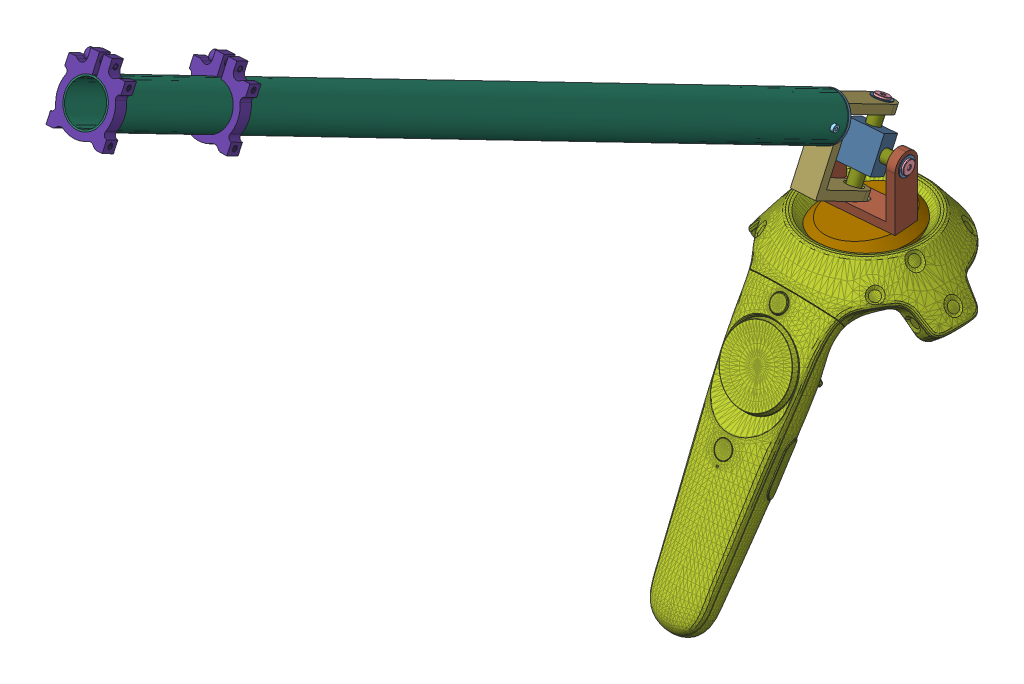
SolidWorks assembly WandMountCAl, configuration Default. Lengths in mm.
Overall size (118.5 507.84 533.23).
33 component instances, 17 part files, 72 mates.
Components (placement in the parent):
- 57155K301_Stainless Steel Ball BearingBAl-5: 57155K301_Stainless Steel Ball BearingBAl [57155K301] at (0 1.0795 0) x (-0.199974 0 0.979801) z (0 1 0) size (10.72 10.72 3.17)
- 57155K301_Stainless Steel Ball BearingBAl-6: 57155K301_Stainless Steel Ball BearingBAl [57155K301] at (0 13.9205 0) x (0.455162 0 -0.890409) z (0 -1 0) size (10.72 10.72 3.17)
- 91251A196_Black-Oxide Alloy Steel Socket Head ScrewAl-1: 91251A196_Black-Oxide Alloy Steel Socket Head ScrewAl [91251A196] at (0 -5.6453 12.5) x (0.587183 0 -0.809454) z (0 -1 0) size (6.86 6.86 20.6)
- 91251A196_Black-Oxide Alloy Steel Socket Head ScrewAl-2: 91251A196_Black-Oxide Alloy Steel Socket Head ScrewAl [91251A196] at (0 -5.6453 -12.5) x (0.424116 0 -0.905608) z (0 -1 0) size (6.86 6.86 20.6)
- 92012A207_Alloy Steel Precision Shoulder ScrewAl-1: 92012A207_Alloy Steel Precision Shoulder ScrewAl [92012A207] at (0 -6.0643 0) x (0.734602 0 0.678499) z (0 -1 0) size (7.94 7.94 28.23)
- 57155K301_Stainless Steel Ball BearingBAl-7: 57155K301_Stainless Steel Ball BearingBAl [57155K301] at (21.3447 48.8017 -1.7999) x (-0.030138 -0.933464 -0.357402) z (-0.996464 0 0.084026) size (10.72 10.72 3.17)
- 57155K301_Stainless Steel Ball BearingBAl-8: 57155K301_Stainless Steel Ball BearingBAl [57155K301] at (0.8273 29.7783 9.8114) x (-0.627222 -0.378377 -0.680752) z (-0.038623 0.888094 -0.458036) size (10.72 10.72 3.17)
- 57155K301_Stainless Steel Ball BearingBAl-9: 57155K301_Stainless Steel Ball BearingBAl [57155K301] at (-21.3447 48.8017 1.7999) x (-0.082588 -0.184207 -0.979412) z (0.996464 0 -0.084026) size (10.72 10.72 3.17)
- 57155K301_Stainless Steel Ball BearingBAl-10: 57155K301_Stainless Steel Ball BearingBAl [57155K301] at (-0.8273 67.8252 -9.8114) x (0.991908 -0.021405 -0.125143) z (0.038623 -0.888094 0.458036) size (10.72 10.72 3.17)
- 90318A302_Ultra-Low-Profile Precision Shoulder ScrewAl-1: 90318A302_Ultra-Low-Profile Precision Shoulder ScrewAl [90318A302] at (-24.113 48.8017 2.0333) x (0.034978 -0.909239 0.414801) z (-0.996464 0 0.084026) size (7.94 7.94 15.93)
- 90318A302_Ultra-Low-Profile Precision Shoulder ScrewAl-2: 90318A302_Ultra-Low-Profile Precision Shoulder ScrewAl [90318A302] at (0.9346 27.3111 11.0839) x (-0.528864 0.370748 0.763445) z (0.038623 -0.888094 0.458036) size (7.94 7.94 15.93)
- 90318A302_Ultra-Low-Profile Precision Shoulder ScrewAl-3: 90318A302_Ultra-Low-Profile Precision Shoulder ScrewAl [90318A302] at (24.113 48.8017 -2.0333) x (0.083807 0.072112 0.993869) z (0.996464 0 -0.084026) size (7.94 7.94 15.93)
- 90318A302_Ultra-Low-Profile Precision Shoulder ScrewAl-4: 90318A302_Ultra-Low-Profile Precision Shoulder ScrewAl [90318A302] at (-0.9346 70.2924 -11.0839) x (0.980778 -0.054045 -0.187492) z (-0.038623 0.888094 -0.458036) size (7.94 7.94 15.93)
- 91290A015_Black-Oxide Alloy Steel Socket Head ScrewAl-1: 91290A015_Black-Oxide Alloy Steel Socket Head ScrewAl [91290A015] at (9.1737 81.0482 32.3414) x (-0.036412 0.683823 -0.728739) z (0.999254 0.034314 -0.017729) size (3.8 3.8 10.09)
- 91290A015_Black-Oxide Alloy Steel Socket Head ScrewAl-2: 91290A015_Black-Oxide Alloy Steel Socket Head ScrewAl [91290A015] at (-10.2118 80.3825 32.6853) x (-0.0328 0.511547 -0.858629) z (-0.999254 -0.034314 0.017729) size (3.8 3.8 10.09)
- 91251A192_Black-Oxide Alloy Steel Socket Head Screw-1: 91251A192_Black-Oxide Alloy Steel Socket Head Screw [91251A192] at (-0.5194 74.5981 20.6527) x (-0.99894 -0.040898 0.021125) z (-0.000028 -0.458379 -0.888757) size (6.86 6.86 14.21)
- Vive Controller 1.5BAl-1: Vive Controller 1.5BAl [Default] at (0.0016 6.0546 36.5874) x (1 -0.000227 0) z (-0.000192 -0.847056 0.531504) size (118.44 84.37 219.45)
- BottomPlugBAl-2: BottomPlugBAl [Default] at origin size (42.24 11.38 42.24)
- TopPlugBAl-2: TopPlugBAl [Default] at origin size (50.17 16.12 56.99)
- CrossAl-1: CrossAl [Default] at (0 48.8017 0) x (-0.996464 0 0.084026) z (0.038623 -0.888094 0.458036) size (20 10 20)
- FORKAl-1: FORKAl [Default] at (0 48.8017 0) x (-0.996464 0 0.084026) z (0 1 0) size (45 15 40)
- ForkTopAl-2: ForkTopAl [Default] at (0 48.8017 0) x (0.038623 -0.888094 0.458036) z (-0.000028 -0.458379 -0.888757) size (45 15 40)
- GimbalSpacerP3BAl-9: GimbalSpacerP3BAl [Default] at (0 -1.3017 0) x (0 1 0) z (0.815244 0 -0.579118) size (0.79 8 8)
- GimbalSpacerP3BAl-10: GimbalSpacerP3BAl [Default] at (0 -2.0955 0) x (0 1 0) z (0.691499 0 -0.722378) size (0.79 8 8)
- GimbalSpacerP3BAl-11: GimbalSpacerP3BAl [Default] at (0 15.508 0) x (0 1 0) z (0.519515 0 -0.854462) size (0.79 8 8)
- GimbalPlugP3CAl-1: GimbalPlugP3CAl [Default] at (-0.5194 75.6617 22.7148) x (-0.999254 -0.034314 0.017729) z (-0.038623 0.888094 -0.458036) size (25.4 16.5 25.4)
- MainTubeP3Al-1: MainTubeP3Al [Default] at (-0.5193 76.5899 24.5146) x (0.999254 0.034314 -0.017729) z (0.000028 0.458379 0.888757) size (25.4 25.4 504.28)
- CrossSpacer-1: CrossSpacer [Default] at (15.0172 48.8017 -1.2663) x (0.996464 0 -0.084026) z (0.084024 -0.005908 0.996446) size (9.53 7.14 7.14)
- CrossSpacer-2: CrossSpacer [Default] at (-15.0172 48.8017 1.2663) x (-0.996464 0 0.084026) z (-0.01061 0.991996 -0.12582) size (9.53 7.14 7.14)
- CrossSpacer-4: CrossSpacer [Default] at (-0.5821 62.1858 -6.9028) x (-0.038623 0.888094 -0.458036) z (0.818712 0.290928 0.495048) size (9.53 7.14 7.14)
- CrossSpacer-6: CrossSpacer [Default] at (0.5821 35.4177 6.9028) x (0.038623 -0.888094 0.458036) z (-0.347024 0.417928 0.839589) size (9.53 7.14 7.14)
- 545680P3-1: 545680P3 [Default] at (-0.1291 309.2768 462.1783) x (-0.999254 -0.034314 0.017729) z (0.038623 -0.888094 0.458036) size (33.53 7.62 39.7)
- 545680P3-2: 545680P3 [Default] at (-0.1315 270.3145 386.634) x (-0.999254 -0.034314 0.017729) z (0.038623 -0.888094 0.458036) size (33.53 7.62 39.7)
Mates (geometry in assembly coordinates):
- Coincident5: coincident aligned: plane of Vive Controller 1.5-1 through (0.0016 0 36.5874) normal (0 1 0)
- Coincident4: coordinate: point of BottomPlug-2
- Coincident6: coincident: line of Vive Controller 1.5-1 through (0 0 0) axis (0 1 0)
- Coincident7: coincident: line of Vive Controller 1.5-1 through (0 0 0) axis (0 1 0)
- Parallel1: parallel anti-aligned: plane of Vive Controller 1.5-1 through (0.0016 6.0546 -0.0032) normal (0 0 -1)
- Coincident9: coordinate: unknown of TopPlugB-2
- Concentric45: concentric aligned: cylinder of 57155K301_Stainless Steel Ball BearingB-5 through (0 1.0795 0) axis (0 1 0) radius 2.3813; cylinder of 92012A207_Alloy Steel Precision Shoulder ScrewAl-1 through (0 21.717 0) axis (0 1 0) radius 2.3813
- Concentric47: concentric anti-aligned: cylinder of 57155K301_Stainless Steel Ball BearingB-6 through (0 13.9205 0) axis (0 -1 0) radius 2.3813; cylinder of 92012A207_Alloy Steel Precision Shoulder ScrewAl-1 through (0 21.717 0) axis (0 1 0) radius 2.3813
- Concentric56: concentric anti-aligned: cylinder of TopPlugB-2 through (0 3.5 0) axis (0 -1 0) radius 4.7625; cylinder of 57155K301_Stainless Steel Ball BearingB-5 through (0 1.0795 0) axis (0 1 0) radius 4.7625
- Coincident41: coincident anti-aligned: plane of TopPlugB-2 through (0 0 0) normal (0 -1 0); plane of 57155K301_Stainless Steel Ball BearingB-5 through (5.2511 0 1.0717) normal (0 1 0)
- Concentric57: concentric anti-aligned: cylinder of TopPlugB-2 through (0 11.5 0) axis (0 1 0) radius 4.7625; cylinder of 57155K301_Stainless Steel Ball BearingB-6 through (0 13.9205 0) axis (0 -1 0) radius 4.7625
- Coincident42: coincident anti-aligned: plane of TopPlugB-2 through (0 15 0) normal (0 1 0); plane of 57155K301_Stainless Steel Ball BearingB-6 through (4.7721 15 2.4394) normal (0 -1 0)
- Concentric63: concentric anti-aligned: cylinder of BottomPlugB-2 through (0 -11.5 12.5) axis (0 -1 0) radius 2.2479; cylinder of 91251A196_Black-Oxide Alloy Steel Socket Head Screw-1 through (0 4.375 12.5) axis (0 1 0) radius 3.429
- Coincident43: coincident anti-aligned: plane of BottomPlugB-2 through (0 -11.5 0) normal (0 -1 0); plane of 91251A196_Black-Oxide Alloy Steel Socket Head Screw-1 through (2.4384 -11.5 14.2689) normal (0 1 0)
- Concentric64: concentric anti-aligned: cylinder of BottomPlugB-2 through (0 -11.5 -12.5) axis (0 -1 0) radius 2.2479; cylinder of 91251A196_Black-Oxide Alloy Steel Socket Head Screw-2 through (0 4.375 -12.5) axis (0 1 0) radius 3.429
- Coincident44: coincident anti-aligned: plane of BottomPlugB-2 through (0 -11.5 0) normal (0 -1 0); plane of 91251A196_Black-Oxide Alloy Steel Socket Head Screw-2 through (2.7281 -11.5 -11.2224) normal (0 1 0)
- Width1: width anti-aligned: plane of FORKAl-1 through (-16.8079 56.3017 8.9439) normal (0.996464 0 -0.084026); plane of FORKAl-1 through (18.0683 21.3018 6.003) normal (-0.996464 0 0.084026); plane of CrossAl-1 through (-10.3377 46.5034 -3.5845) normal (-0.996464 0 0.084026); plane of CrossAl-1 through (9.5915 46.5034 -5.265) normal (0.996464 0 -0.084026)
- Width2: width aligned: plane of ForkTopAl-2 through (-8.1695 76.6915 16.5581) normal (0.038623 -0.888094 0.458036); plane of ForkTopAl-2 through (-6.8187 29.5649 1.4829) normal (-0.038623 0.888094 -0.458036); plane of CrossAl-1 through (0.0131 37.6225 0.1556) normal (0.038623 -0.888094 0.458036); plane of CrossAl-1 through (-0.7593 55.3844 -9.0051) normal (-0.038623 0.888094 -0.458036)
- Concentric7: concentric aligned: cylinder of FORKAl-1 through (22.4204 48.8017 -1.8906) axis (-0.996464 0 0.084026) radius 4.7625; cylinder of 57155K301_Stainless Steel Ball BearingBAl-7 through (21.3447 48.8017 -1.7999) axis (-0.996464 0 0.084026) radius 4.7625
- Coincident10: coincident anti-aligned: plane of FORKAl-1 through (23.0506 56.3017 5.5829) normal (0.996464 0 -0.084026); plane of 57155K301_Stainless Steel Ball BearingBAl-7 through (22.8408 46.8795 3.0945) normal (-0.996464 0 0.084026)
- Concentric9: concentric anti-aligned: cylinder of FORKAl-1 through (22.4204 48.8017 -1.8906) axis (-0.996464 0 0.084026) radius 4.7625; cylinder of 57155K301_Stainless Steel Ball BearingBAl-9 through (-21.3447 48.8017 1.7999) axis (0.996464 0 -0.084026) radius 4.7625
- Coincident12: coincident anti-aligned: plane of FORKAl-1 through (-21.7902 16.3018 9.3641) normal (-0.996464 0 0.084026); plane of 57155K301_Stainless Steel Ball BearingBAl-9 through (-22.5034 54.0694 0.9068) normal (0.996464 0 -0.084026)
- Concentric8: concentric anti-aligned: cylinder of ForkTopAl-2 through (-0.869 68.7839 -10.3058) axis (0.038623 -0.888094 0.458036) radius 4.7625; cylinder of 57155K301_Stainless Steel Ball BearingBAl-8 through (0.8273 29.7783 9.8114) axis (-0.038623 0.888094 -0.458036) radius 4.7625
- Coincident11: coincident anti-aligned: plane of ForkTopAl-2 through (-6.6245 43.4596 39.3234) normal (0.038623 -0.888094 0.458036); plane of 57155K301_Stainless Steel Ball BearingBAl-8 through (-3.3 30.2184 13.3695) normal (-0.038623 0.888094 -0.458036)
- Concentric10: concentric aligned: cylinder of ForkTopAl-2 through (-0.869 68.7839 -10.3058) axis (0.038623 -0.888094 0.458036) radius 4.7625; cylinder of 57155K301_Stainless Steel Ball BearingBAl-10 through (-0.8273 67.8252 -9.8114) axis (0.038623 -0.888094 0.458036) radius 4.7625
- Coincident13: coincident anti-aligned: plane of ForkTopAl-2 through (-8.3636 65.0887 -16.8385) normal (-0.038623 0.888094 -0.458036); plane of 57155K301_Stainless Steel Ball BearingBAl-10 through (-0.2208 71.2447 -5.5891) normal (0.038623 -0.888094 0.458036)
- Concentric15: concentric aligned: cylinder of 57155K301_Stainless Steel Ball BearingBAl-7 through (21.3447 48.8017 -1.7999) axis (-0.996464 0 0.084026) radius 2.3813; cylinder of 90318A302_Ultra-Low-Profile Precision Shoulder ScrewAl-3 through (8.6897 48.8017 -0.7327) axis (-0.996464 0 0.084026) radius 2.3813
- Coincident16: coincident anti-aligned: plane of 57155K301_Stainless Steel Ball BearingBAl-7 through (23.1694 47.6914 0.9462) normal (0.996464 0 -0.084026); plane of 90318A302_Ultra-Low-Profile Precision Shoulder ScrewAl-3 through (22.9026 52.7602 -2.2184) normal (-0.996464 0 0.084026)
- Concentric13: concentric aligned: cylinder of 57155K301_Stainless Steel Ball BearingBAl-8 through (0.8273 29.7783 9.8114) axis (-0.038623 0.888094 -0.458036) radius 2.3813; cylinder of 90318A302_Ultra-Low-Profile Precision Shoulder ScrewAl-2 through (0.3368 41.0571 3.9943) axis (-0.038623 0.888094 -0.458036) radius 2.3813
- Coincident15: coincident anti-aligned: plane of 57155K301_Stainless Steel Ball BearingBAl-8 through (-1.5194 29.1764 12.3081) normal (0.038623 -0.888094 0.458036); plane of 90318A302_Ultra-Low-Profile Precision Shoulder ScrewAl-2 through (4.2535 29.4469 12.3457) normal (-0.038623 0.888094 -0.458036)
- Concentric11: concentric aligned: cylinder of 57155K301_Stainless Steel Ball BearingBAl-9 through (-21.3447 48.8017 1.7999) axis (0.996464 0 -0.084026) radius 2.3813; cylinder of 90318A302_Ultra-Low-Profile Precision Shoulder ScrewAl-1 through (-8.6897 48.8017 0.7327) axis (0.996464 0 -0.084026) radius 2.3813
- Coincident14: coincident anti-aligned: plane of 57155K301_Stainless Steel Ball BearingBAl-9 through (-22.9745 51.8444 1.365) normal (-0.996464 0 0.084026); plane of 90318A302_Ultra-Low-Profile Precision Shoulder ScrewAl-1 through (-23.2298 47.1497 -1.6625) normal (0.996464 0 -0.084026)
- Concentric17: concentric aligned: cylinder of 57155K301_Stainless Steel Ball BearingBAl-10 through (-0.8273 67.8252 -9.8114) axis (0.038623 -0.888094 0.458036) radius 2.3813; cylinder of 90318A302_Ultra-Low-Profile Precision Shoulder ScrewAl-4 through (-0.3368 56.5464 -3.9943) axis (0.038623 -0.888094 0.458036) radius 2.3813
- Coincident17: coincident anti-aligned: plane of 57155K301_Stainless Steel Ball BearingBAl-10 through (-0.5143 70.6564 -7.8141) normal (-0.038623 0.888094 -0.458036); plane of 90318A302_Ultra-Low-Profile Precision Shoulder ScrewAl-4 through (-0.1296 71.0466 -7.0899) normal (0.038623 -0.888094 0.458036)
- Concentric68: concentric anti-aligned: cylinder of 92012A207_Alloy Steel Precision Shoulder ScrewAl-1 through (0 21.717 0) axis (0 1 0) radius 2.3813; cylinder of GimbalSpacerP3BAl-9 through (0 -0.508 0) axis (0 -1 0) radius 2.3813
- Coincident48: coincident anti-aligned: plane of 57155K301_Stainless Steel Ball BearingB-5 through (3.0331 -0.508 0.619) normal (0 -1 0); plane of GimbalSpacerP3BAl-9 through (0 -0.508 0) normal (0 1 0)
- Concentric69: concentric anti-aligned: cylinder of 92012A207_Alloy Steel Precision Shoulder ScrewAl-1 through (0 21.717 0) axis (0 1 0) radius 2.3813; cylinder of GimbalSpacerP3BAl-10 through (0 -1.3017 0) axis (0 -1 0) radius 2.3813
- Coincident49: coincident anti-aligned: plane of GimbalSpacerP3BAl-9 through (0 -1.3017 0) normal (0 -1 0); plane of GimbalSpacerP3BAl-10 through (0 -1.3017 0) normal (0 1 0)
- Concentric70: concentric anti-aligned: cylinder of 92012A207_Alloy Steel Precision Shoulder ScrewAl-1 through (0 21.717 0) axis (0 1 0) radius 2.3813; cylinder of GimbalSpacerP3BAl-11 through (0 16.3018 0) axis (0 -1 0) radius 2.3813
- Coincident51: coincident anti-aligned: plane of 92012A207_Alloy Steel Precision Shoulder ScrewAl-1 through (2.6928 -2.0955 -2.9155) normal (0 1 0); plane of GimbalSpacerP3BAl-10 through (0 -2.0955 0) normal (0 -1 0)
- Coincident52: coincident anti-aligned: plane of 57155K301_Stainless Steel Ball BearingB-6 through (2.7564 15.508 1.409) normal (0 1 0); plane of GimbalSpacerP3BAl-11 through (0 15.508 0) normal (0 -1 0)
- Coincident56: coincident anti-aligned: plane of ForkTopAl-2 through (-8.3625 83.4238 18.7117) normal (0.000028 0.458379 0.888757); plane of GimbalPlugP3CAl-1 through (-1.0099 86.9405 16.8978) normal (-0.000028 -0.458379 -0.888757)
- Coincident62: coincident aligned: axis of 91290A015_Black-Oxide Alloy Steel Socket Head ScrewAl-2 through (-13.2096 80.2796 32.7385) axis (0.999254 0.034314 -0.017729); line of MainTubeP3Al-1 through (-13.2096 80.2796 32.7385) axis (0.999254 0.034314 -0.017729)
- Coincident63: coincident aligned: line of GimbalPlugP3CAl-1 through (-0.5189 83.225 37.3793) axis (-0.000028 -0.458379 -0.888757); line of MainTubeP3Al-1 through (-0.5052 307.7415 472.6967) axis (-0.000028 -0.458379 -0.888757)
- Tangent4: tangent anti-aligned: plane of 91290A015_Black-Oxide Alloy Steel Socket Head ScrewAl-1 through (12.1483 82.463 33.5204) normal (-0.999254 -0.034314 0.017729); cylinder of MainTubeP3Al-1 through (-0.5052 307.7415 472.6967) axis (-0.000028 -0.458379 -0.888757) radius 12.7
- Tangent5: tangent anti-aligned: plane of 91290A015_Black-Oxide Alloy Steel Socket Head ScrewAl-2 through (-13.1729 78.7341 31.8164) normal (0.999254 0.034314 -0.017729); cylinder of MainTubeP3Al-1 through (-0.5052 307.7415 472.6967) axis (-0.000028 -0.458379 -0.888757) radius 12.7
- Concentric73: concentric anti-aligned: cylinder of 90318A302_Ultra-Low-Profile Precision Shoulder ScrewAl-1 through (-8.6897 48.8017 0.7327) axis (0.996464 0 -0.084026) radius 2.3813; cylinder of CrossAl-1 through (-9.9646 48.8017 0.8403) axis (-0.996464 0 0.084026) radius 1.7272
- Concentric74: concentric anti-aligned: cylinder of 90318A302_Ultra-Low-Profile Precision Shoulder ScrewAl-3 through (8.6897 48.8017 -0.7327) axis (-0.996464 0 0.084026) radius 2.3813; cylinder of CrossAl-1 through (9.9646 48.8017 -0.8403) axis (0.996464 0 -0.084026) radius 1.7272
- Concentric75: concentric anti-aligned: cylinder of 90318A302_Ultra-Low-Profile Precision Shoulder ScrewAl-2 through (0.3368 41.0571 3.9943) axis (-0.038623 0.888094 -0.458036) radius 2.3813; cylinder of CrossAl-1 through (0.3862 39.9208 4.5804) axis (0.038623 -0.888094 0.458036) radius 1.7272
- Concentric76: concentric anti-aligned: cylinder of 90318A302_Ultra-Low-Profile Precision Shoulder ScrewAl-4 through (-0.3368 56.5464 -3.9943) axis (0.038623 -0.888094 0.458036) radius 2.3813; cylinder of CrossAl-1 through (-0.3862 57.6827 -4.5804) axis (-0.038623 0.888094 -0.458036) radius 1.7272
- Concentric77: concentric aligned: cylinder of ForkTopAl-2 through (-0.5195 73.3698 18.2711) axis (-0.000028 -0.458379 -0.888757) radius 1.7272; cylinder of GimbalPlugP3CAl-1 through (-0.5472 -382.7178 -866.0417) axis (-0.000028 -0.458379 -0.888757) radius 2.8067
- Concentric78: concentric anti-aligned: cylinder of GimbalPlugP3CAl-1 through (-11.6233 80.334 32.7104) axis (-0.999254 -0.034314 0.017729) radius 1.25; cylinder of 91290A015_Black-Oxide Alloy Steel Socket Head ScrewAl-2 through (-5.2155 80.5541 32.5967) axis (0.999254 0.034314 -0.017729) radius 1.9
- Concentric79: concentric anti-aligned: cylinder of GimbalPlugP3CAl-1 through (10.5852 81.0967 32.3164) axis (0.999254 0.034314 -0.017729) radius 1.25; cylinder of 91290A015_Black-Oxide Alloy Steel Socket Head ScrewAl-1 through (4.1774 80.8766 32.4301) axis (-0.999254 -0.034314 0.017729) radius 1.9
- Parallel3: parallel aligned: plane of ForkTopAl-2 through (-8.3636 65.0887 -16.8385) normal (-0.038623 0.888094 -0.458036); plane of GimbalPlugP3CAl-1 through (-0.5194 75.6617 22.7148) normal (-0.038623 0.888094 -0.458036)
- Concentric80: concentric anti-aligned: cylinder of ForkTopAl-2 through (-0.5195 73.3698 18.2711) axis (-0.000028 -0.458379 -0.888757) radius 1.7272; cylinder of 91251A192_Black-Oxide Alloy Steel Socket Head Screw-1 through (-0.5192 77.7359 26.7365) axis (0.000028 0.458379 0.888757) radius 3.429
- Coincident64: coincident anti-aligned: plane of ForkTopAl-2 through (-6.8177 45.6082 32.5894) normal (-0.000028 -0.458379 -0.888757); plane of 91251A192_Black-Oxide Alloy Steel Socket Head Screw-1 through (-0.6582 76.0443 16.8917) normal (0.000028 0.458379 0.888757)
- Concentric81: concentric aligned: cylinder of 90318A302_Ultra-Low-Profile Precision Shoulder ScrewAl-3 through (8.6897 48.8017 -0.7327) axis (-0.996464 0 0.084026) radius 2.3813; cylinder of CrossSpacer-1 through (19.7629 48.8017 -1.6665) axis (-0.996464 0 0.084026) radius 2.3813
- Coincident65: coincident anti-aligned: plane of 57155K301_Stainless Steel Ball BearingBAl-7 through (19.9496 47.9477 0.5485) normal (-0.996464 0 0.084026); plane of CrossSpacer-1 through (19.7629 48.8017 -1.6665) normal (0.996464 0 -0.084026)
- Concentric82: concentric aligned: cylinder of 90318A302_Ultra-Low-Profile Precision Shoulder ScrewAl-1 through (-8.6897 48.8017 0.7327) axis (0.996464 0 -0.084026) radius 2.3813; cylinder of CrossSpacer-2 through (-19.7629 48.8017 1.6665) axis (0.996464 0 -0.084026) radius 2.3813
- Coincident66: coincident anti-aligned: plane of 57155K301_Stainless Steel Ball BearingBAl-9 through (-19.7997 51.1423 1.2294) normal (0.996464 0 -0.084026); plane of CrossSpacer-2 through (-19.7629 48.8017 1.6665) normal (-0.996464 0 0.084026)
- Concentric83: concentric aligned: cylinder of 90318A302_Ultra-Low-Profile Precision Shoulder ScrewAl-4 through (-0.3368 56.5464 -3.9943) axis (0.038623 -0.888094 0.458036) radius 2.3813; cylinder of CrossSpacer-4 through (-0.766 66.4153 -9.0842) axis (0.038623 -0.888094 0.458036) radius 2.3813
- Coincident67: coincident anti-aligned: plane of 57155K301_Stainless Steel Ball BearingBAl-10 through (-0.478 67.5087 -6.9885) normal (0.038623 -0.888094 0.458036); plane of CrossSpacer-4 through (-0.766 66.4153 -9.0842) normal (-0.038623 0.888094 -0.458036)
- Concentric84: concentric aligned: cylinder of 90318A302_Ultra-Low-Profile Precision Shoulder ScrewAl-2 through (0.3368 41.0571 3.9943) axis (-0.038623 0.888094 -0.458036) radius 2.3813; cylinder of CrossSpacer-6 through (0.766 31.1882 9.0842) axis (-0.038623 0.888094 -0.458036) radius 2.3813
- Coincident68: coincident anti-aligned: plane of 57155K301_Stainless Steel Ball BearingBAl-8 through (-1.0863 31.8097 10.4455) normal (-0.038623 0.888094 -0.458036); plane of CrossSpacer-6 through (0.766 31.1882 9.0842) normal (0.038623 -0.888094 0.458036)
- Concentric85: concentric anti-aligned: cylinder of MainTubeP3Al-1 through (-0.5052 307.7415 472.6967) axis (-0.000028 -0.458379 -0.888757) radius 12.7; cylinder of 545680P3-1 through (-0.5054 304.2487 465.9244) axis (0.000028 0.458379 0.888757) radius 12.5
- Coincident69: coincident aligned: plane of MainTubeP3Al-1 through (-0.5052 307.7415 472.6967) normal (0.000028 0.458379 0.888757); plane of 545680P3-1 through (-13.4446 295.317 479.1051) normal (0.000028 0.458379 0.888757)
- Parallel4: parallel anti-aligned: plane of MainTubeP3Al-1 through (-0.5193 76.5899 24.5146) normal (0.999254 0.034314 -0.017729); plane of 545680P3-1 through (-0.1291 309.2768 462.1783) normal (-0.999254 -0.034314 0.017729)
- Concentric86: concentric anti-aligned: cylinder of MainTubeP3Al-1 through (-0.5052 307.7415 472.6967) axis (-0.000028 -0.458379 -0.888757) radius 12.7; cylinder of 545680P3-2 through (-0.5078 265.2864 390.3801) axis (0.000028 0.458379 0.888757) radius 12.5
- Parallel5: parallel anti-aligned: plane of MainTubeP3Al-1 through (-0.5193 76.5899 24.5146) normal (0.999254 0.034314 -0.017729); plane of 545680P3-2 through (-0.1315 270.3145 386.634) normal (-0.999254 -0.034314 0.017729)
- Distance1: distance = 85 mm aligned: plane of 545680P3-1 through (-13.4448 291.8242 472.3328) normal (-0.000028 -0.458379 -0.888757); plane of 545680P3-2 through (-13.4471 252.8619 396.7885) normal (-0.000028 -0.458379 -0.888757)
- Coincident70: coincident anti-aligned: plane of FORKAl-1 through (23.0506 16.3018 5.5829) normal (0 -1 0); plane of GimbalSpacerP3BAl-11 through (0 16.3018 0) normal (0 1 0)
- Concentric87: concentric aligned: cylinder of 92012A207_Alloy Steel Precision Shoulder ScrewAl-1 through (0 21.717 0) axis (0 1 0) radius 2.3813; cylinder of FORKAl-1 through (0 21.3018 0) axis (0 1 0) radius 1.7272
